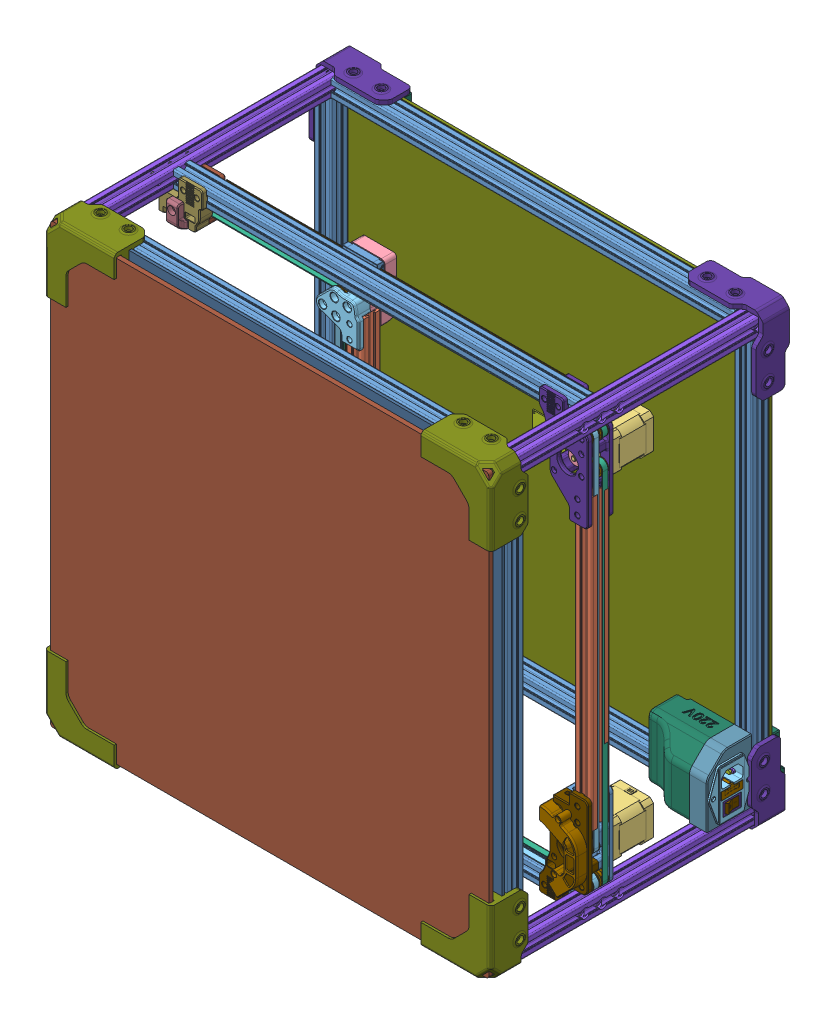
SolidWorks assembly Assem, configuration Default. Lengths in mm. (continued)
Mates (geometry in assembly coordinates): (continued)
- Coincident18: coincident anti-aligned: plane of F695 ZZ (1)^Idler Assembly (1)_1_XY Joint - Right_X Axis_Gantry_VORON2 v2.4 Assembly - Final(2)_VORON2 v2.4 Assembly - Final-1 through (-40.7546 -221.05 -5.3) normal (0 0 1); plane of F695 ZZ (1)^Idler Assembly (1)_1_XY Joint - Right_X Axis_Gantry_VORON2 v2.4 Assembly - Final(2)_VORON2 v2.4 Assembly - Final-2 through (-40.7546 -221.05 -5.3) normal (0 0 -1)
- Concentric9: concentric anti-aligned: cylinder of F695 ZZ (1)^Idler Assembly (1)_1_XY Joint - Right_X Axis_Gantry_VORON2 v2.4 Assembly - Final(2)_VORON2 v2.4 Assembly - Final-1 through (-40.7546 -221.05 -7.3) axis (0 0 1) radius 6.5; cylinder of F695 ZZ (1)^Idler Assembly (1)_1_XY Joint - Right_X Axis_Gantry_VORON2 v2.4 Assembly - Final(2)_VORON2 v2.4 Assembly - Final-2 through (-40.7546 -221.05 -3.3) axis (0 0 -1) radius 6.5
- Concentric10: concentric anti-aligned: cylinder of XY Joint - Right-63^XY Joint - Right_X Axis_Gantry_VORON2 v2.4 Assembly - Final(2)_VORON2 v2.4 Assembly - Final-1 through (-40.7546 -221.05 10.9) axis (0 0 -1) radius 2.7; cylinder of F695 ZZ (1)^Idler Assembly (1)_1_XY Joint - Right_X Axis_Gantry_VORON2 v2.4 Assembly - Final(2)_VORON2 v2.4 Assembly - Final-2 through (-40.7546 -221.05 -5.3) axis (0 0 1) radius 2.5
- Distance7: distance = 1 mm anti-aligned: plane of F695 ZZ (1)^Idler Assembly (1)_1_XY Joint - Right_X Axis_Gantry_VORON2 v2.4 Assembly - Final(2)_VORON2 v2.4 Assembly - Final-1 through (-40.7546 -221.05 -9.3) normal (0 0 -1); plane of XY Joint - Right-63^XY Joint - Right_X Axis_Gantry_VORON2 v2.4 Assembly - Final(2)_VORON2 v2.4 Assembly - Final-1 through (-40.1448 -212.776 -10.3) normal (0 0 1)
- Coincident20: coincident anti-aligned: plane of XY Joint - Right-63^XY Joint - Right_X Axis_Gantry_VORON2 v2.4 Assembly - Final(2)_VORON2 v2.4 Assembly - Final-1 through (-40.1448 -212.776 -10.3) normal (0 0 1); plane of M5 1mm Spacer (1)^Idler Assembly (1)_1_XY Joint - Right_X Axis_Gantry_VORON2 v2.4 Assembly - Final(2)_VORON2 v2.4 Assembly - Final-1 through (-40.7546 -221.05 -10.3) normal (0 0 -1)
- Concentric13: concentric anti-aligned: cylinder of F695 ZZ (1)^Idler Assembly (1)_1_XY Joint - Right_X Axis_Gantry_VORON2 v2.4 Assembly - Final(2)_VORON2 v2.4 Assembly - Final-1 through (-40.7546 -221.05 -9.3) axis (0 0 1) radius 7.5; cylinder of M5 1mm Spacer (1)^Idler Assembly (1)_1_XY Joint - Right_X Axis_Gantry_VORON2 v2.4 Assembly - Final(2)_VORON2 v2.4 Assembly - Final-1 through (-40.7546 -221.05 -9.3) axis (0 0 -1) radius 5
- Coincident21: coincident anti-aligned: plane of F695 ZZ (1)^Idler Assembly (1)_1_XY Joint - Right_X Axis_Gantry_VORON2 v2.4 Assembly - Final(2)_VORON2 v2.4 Assembly - Final-2 through (-40.7546 -221.05 -1.3) normal (0 0 1); plane of M5 1mm Spacer (1)^Idler Assembly (1)_1_XY Joint - Right_X Axis_Gantry_VORON2 v2.4 Assembly - Final(2)_VORON2 v2.4 Assembly - Final-2 through (-40.7546 -221.05 -1.3) normal (0 0 -1)
- Concentric14: concentric aligned: cylinder of F695 ZZ (1)^Idler Assembly (1)_1_XY Joint - Right_X Axis_Gantry_VORON2 v2.4 Assembly - Final(2)_VORON2 v2.4 Assembly - Final-2 through (-40.7546 -221.05 -1.3) axis (0 0 -1) radius 7.5; cylinder of M5 1mm Spacer (1)^Idler Assembly (1)_1_XY Joint - Right_X Axis_Gantry_VORON2 v2.4 Assembly - Final(2)_VORON2 v2.4 Assembly - Final-2 through (-40.7546 -221.05 -0.3) axis (0 0 -1) radius 5
- Distance8: distance = 250 mm aligned: plane of ALP2020_460-1 through (230 250 8.5) normal (0 1 0)
- Coincident23: coincident aligned: plane of ALP2020_460-1 through (0 240 0) normal (1 0 0)
- Coincident24: coincident aligned: plane of ALP2020_460-1 through (0 240 0) normal (0 0 1)
- Concentric15: concentric anti-aligned: cylinder of F695 ZZ (1)^Idler Assembly (1)_1_XY Joint - Right_X Axis_Gantry_VORON2 v2.4 Assembly - Final(2)_VORON2 v2.4 Assembly - Final-3 through (-40.7546 221.05 6.7) axis (0 0 -1) radius 6.5; cylinder of F695 ZZ (1)^Idler Assembly (1)_1_XY Joint - Right_X Axis_Gantry_VORON2 v2.4 Assembly - Final(2)_VORON2 v2.4 Assembly - Final-4 through (-40.7546 221.05 2.7) axis (0 0 1) radius 6.5
- Coincident25: coincident anti-aligned: plane of F695 ZZ (1)^Idler Assembly (1)_1_XY Joint - Right_X Axis_Gantry_VORON2 v2.4 Assembly - Final(2)_VORON2 v2.4 Assembly - Final-3 through (-40.7546 221.05 4.7) normal (0 0 -1); plane of F695 ZZ (1)^Idler Assembly (1)_1_XY Joint - Right_X Axis_Gantry_VORON2 v2.4 Assembly - Final(2)_VORON2 v2.4 Assembly - Final-4 through (-40.7546 221.05 4.7) normal (0 0 1)
- Concentric16: concentric anti-aligned: cylinder of M5 1mm Spacer (1)^Idler Assembly (1)_1_XY Joint - Right_X Axis_Gantry_VORON2 v2.4 Assembly - Final(2)_VORON2 v2.4 Assembly - Final-4 through (-40.7546 221.05 0.7) axis (0 0 -1) radius 5; cylinder of F695 ZZ (1)^Idler Assembly (1)_1_XY Joint - Right_X Axis_Gantry_VORON2 v2.4 Assembly - Final(2)_VORON2 v2.4 Assembly - Final-4 through (-40.7546 221.05 0.7) axis (0 0 1) radius 7.5
- Concentric17: concentric aligned: cylinder of M5 1mm Spacer (1)^Idler Assembly (1)_1_XY Joint - Right_X Axis_Gantry_VORON2 v2.4 Assembly - Final(2)_VORON2 v2.4 Assembly - Final-3 through (-40.7546 221.05 9.7) axis (0 0 -1) radius 5; cylinder of F695 ZZ (1)^Idler Assembly (1)_1_XY Joint - Right_X Axis_Gantry_VORON2 v2.4 Assembly - Final(2)_VORON2 v2.4 Assembly - Final-3 through (-40.7546 221.05 8.7) axis (0 0 -1) radius 7.5
- Coincident26: coincident anti-aligned: plane of M5 1mm Spacer (1)^Idler Assembly (1)_1_XY Joint - Right_X Axis_Gantry_VORON2 v2.4 Assembly - Final(2)_VORON2 v2.4 Assembly - Final-3 through (-40.7546 221.05 8.7) normal (0 0 -1); plane of F695 ZZ (1)^Idler Assembly (1)_1_XY Joint - Right_X Axis_Gantry_VORON2 v2.4 Assembly - Final(2)_VORON2 v2.4 Assembly - Final-3 through (-40.7546 221.05 8.7) normal (0 0 1)
- Concentric18: concentric anti-aligned: cylinder of XY Joint - Left-57^XY Joint - Left_X Axis_Gantry_VORON2 v2.4 Assembly - Final(2)_VORON2 v2.4 Assembly - Final-1 through (-40.7546 221.05 15.7) axis (0 0 1) radius 4.4; cylinder of F695 ZZ (1)^Idler Assembly (1)_1_XY Joint - Right_X Axis_Gantry_VORON2 v2.4 Assembly - Final(2)_VORON2 v2.4 Assembly - Final-4 through (-40.7546 221.05 4.7) axis (0 0 -1) radius 2.5
- Coincident27: coincident anti-aligned: plane of XY Joint - Left-57^XY Joint - Left_X Axis_Gantry_VORON2 v2.4 Assembly - Final(2)_VORON2 v2.4 Assembly - Final-1 through (-42.8669 212.651 9.7) normal (0 0 -1); plane of M5 1mm Spacer (1)^Idler Assembly (1)_1_XY Joint - Right_X Axis_Gantry_VORON2 v2.4 Assembly - Final(2)_VORON2 v2.4 Assembly - Final-3 through (-40.7546 221.05 9.7) normal (0 0 1)
- Coincident28: coincident anti-aligned: plane of M5 1mm Spacer (1)^Idler Assembly (1)_1_XY Joint - Right_X Axis_Gantry_VORON2 v2.4 Assembly - Final(2)_VORON2 v2.4 Assembly - Final-4 through (-40.7546 221.05 0.7) normal (0 0 1); plane of F695 ZZ (1)^Idler Assembly (1)_1_XY Joint - Right_X Axis_Gantry_VORON2 v2.4 Assembly - Final(2)_VORON2 v2.4 Assembly - Final-4 through (-40.7546 221.05 0.7) normal (0 0 -1)
- Coincident29: coincident anti-aligned: plane of Front Idler B Bottom^Front Idler B_Gantry_VORON2 v2.4 Assembly - Final(2)_VORON2 v2.4 Assembly - Final-1 through (-218.2501 228 0) normal (0 0 1); plane of Front Idler B Top^Front Idler B_Gantry_VORON2 v2.4 Assembly - Final(2)_VORON2 v2.4 Assembly - Final-1 through (-207 239.4979 0) normal (0 0 -1)
- Coincident31: coincident aligned: plane of Front Idler B Bottom^Front Idler B_Gantry_VORON2 v2.4 Assembly - Final(2)_VORON2 v2.4 Assembly - Final-1 through (-211.5 218.8388 -15) normal (1 0 0); plane of Front Idler B Top^Front Idler B_Gantry_VORON2 v2.4 Assembly - Final(2)_VORON2 v2.4 Assembly - Final-1 through (-211.5 218.8388 -15) normal (1 0 0)
- Coincident33: coincident anti-aligned: plane of ALP2020_450-1 through (230 231.5 10) normal (0 0 1); plane of Front Idler B Top^Front Idler B_Gantry_VORON2 v2.4 Assembly - Final(2)_VORON2 v2.4 Assembly - Final-1 through (-208.3 228 10) normal (0 0 -1)
- Distance9: distance = 10 mm aligned: plane of Front Idler B Top^Front Idler B_Gantry_VORON2 v2.4 Assembly - Final(2)_VORON2 v2.4 Assembly - Final-1 through (-220 229 10) normal (-1 0 0); plane of ALP2020_450-1 through (-230 245.9 -2.0109) normal (-1 0 0)
- Coincident35: coincident aligned: plane of ALP2020_450-1 through (230 250 8.5) normal (0 1 0); plane of Front Idler B Top^Front Idler B_Gantry_VORON2 v2.4 Assembly - Final(2)_VORON2 v2.4 Assembly - Final-1 through (-221.6 250 10) normal (0 1 0)
- Coincident36: coincident aligned: plane of Front Idler B Bottom^Front Idler B_Gantry_VORON2 v2.4 Assembly - Final(2)_VORON2 v2.4 Assembly - Final-1 through (-221.6 250 -15) normal (0 1 0); plane of Front Idler B Top^Front Idler B_Gantry_VORON2 v2.4 Assembly - Final(2)_VORON2 v2.4 Assembly - Final-1 through (-221.6 250 10) normal (0 1 0)
- Coincident38: coincident anti-aligned: plane of F695 ZZ (1)^Idler Assembly (1)_1_XY Joint - Right_X Axis_Gantry_VORON2 v2.4 Assembly - Final(2)_VORON2 v2.4 Assembly - Final-5 through (-219.5002 221.0003 -5) normal (0 0 -1); plane of F695 ZZ (1)^Idler Assembly (1)_1_XY Joint - Right_X Axis_Gantry_VORON2 v2.4 Assembly - Final(2)_VORON2 v2.4 Assembly - Final-6 through (-219.5002 221.0003 -5) normal (0 0 1)
- Concentric23: concentric anti-aligned: cylinder of F695 ZZ (1)^Idler Assembly (1)_1_XY Joint - Right_X Axis_Gantry_VORON2 v2.4 Assembly - Final(2)_VORON2 v2.4 Assembly - Final-5 through (-219.5002 221.0003 -3) axis (0 0 -1) radius 6.5; cylinder of F695 ZZ (1)^Idler Assembly (1)_1_XY Joint - Right_X Axis_Gantry_VORON2 v2.4 Assembly - Final(2)_VORON2 v2.4 Assembly - Final-6 through (-219.5002 221.0003 -7) axis (0 0 1) radius 6.5
- Concentric24: concentric anti-aligned: cylinder of F695 ZZ (1)^Idler Assembly (1)_1_XY Joint - Right_X Axis_Gantry_VORON2 v2.4 Assembly - Final(2)_VORON2 v2.4 Assembly - Final-5 through (-219.5002 221.0003 -1) axis (0 0 -1) radius 7.5; cylinder of M5 1mm Spacer (1)^Idler Assembly (1)_1_XY Joint - Right_X Axis_Gantry_VORON2 v2.4 Assembly - Final(2)_VORON2 v2.4 Assembly - Final-6 through (-219.5002 221.0003 -1) axis (0 0 1) radius 5
- Coincident39: coincident anti-aligned: plane of F695 ZZ (1)^Idler Assembly (1)_1_XY Joint - Right_X Axis_Gantry_VORON2 v2.4 Assembly - Final(2)_VORON2 v2.4 Assembly - Final-5 through (-219.5002 221.0003 -1) normal (0 0 1); plane of M5 1mm Spacer (1)^Idler Assembly (1)_1_XY Joint - Right_X Axis_Gantry_VORON2 v2.4 Assembly - Final(2)_VORON2 v2.4 Assembly - Final-6 through (-219.5002 221.0003 -1) normal (0 0 -1)
- Coincident40: coincident anti-aligned: plane of M5 1mm Spacer (1)^Idler Assembly (1)_1_XY Joint - Right_X Axis_Gantry_VORON2 v2.4 Assembly - Final(2)_VORON2 v2.4 Assembly - Final-5 through (-219.5002 221.0003 -9) normal (0 0 1); plane of F695 ZZ (1)^Idler Assembly (1)_1_XY Joint - Right_X Axis_Gantry_VORON2 v2.4 Assembly - Final(2)_VORON2 v2.4 Assembly - Final-6 through (-219.5002 221.0003 -9) normal (0 0 -1)
- Concentric25: concentric aligned: cylinder of M5 1mm Spacer (1)^Idler Assembly (1)_1_XY Joint - Right_X Axis_Gantry_VORON2 v2.4 Assembly - Final(2)_VORON2 v2.4 Assembly - Final-5 through (-219.5002 221.0003 -10) axis (0 0 1) radius 5; cylinder of F695 ZZ (1)^Idler Assembly (1)_1_XY Joint - Right_X Axis_Gantry_VORON2 v2.4 Assembly - Final(2)_VORON2 v2.4 Assembly - Final-6 through (-219.5002 221.0003 -9) axis (0 0 1) radius 7.5
- Concentric26: concentric anti-aligned: cylinder of Tensioner B-26^Tensioner B_Front Idler B_Gantry_VORON2 v2.4 Assembly - Final(2)_VORON2 v2.4 Assembly - Final-1 through (-219.5002 221.0003 -15) axis (0 0 1) radius 2.7; cylinder of F695 ZZ (1)^Idler Assembly (1)_1_XY Joint - Right_X Axis_Gantry_VORON2 v2.4 Assembly - Final(2)_VORON2 v2.4 Assembly - Final-6 through (-219.5002 221.0003 -5) axis (0 0 -1) radius 2.5
- Coincident42: coincident anti-aligned: plane of Front Idler A Bottom (1)^Front Idler A_Gantry_VORON2 v2.4 Assembly - Final(2)_VORON2 v2.4 Assembly - Final-1 through (-244.5002 -212 0) normal (0 0 1); plane of Front Idler A Top^Front Idler A_Gantry_VORON2 v2.4 Assembly - Final(2)_VORON2 v2.4 Assembly - Final-1 through (-218.2501 -228 0) normal (0 0 -1)
- Coincident43: coincident aligned: plane of Front Idler A Bottom (1)^Front Idler A_Gantry_VORON2 v2.4 Assembly - Final(2)_VORON2 v2.4 Assembly - Final-1 through (-221.6 -250 -15) normal (0 -1 0); plane of Front Idler A Top^Front Idler A_Gantry_VORON2 v2.4 Assembly - Final(2)_VORON2 v2.4 Assembly - Final-1 through (-221.6 -250 10) normal (0 -1 0)
- Coincident44: coincident aligned: plane of Front Idler A Bottom (1)^Front Idler A_Gantry_VORON2 v2.4 Assembly - Final(2)_VORON2 v2.4 Assembly - Final-1 through (-220 -229 -15) normal (-1 0 0); plane of Front Idler A Top^Front Idler A_Gantry_VORON2 v2.4 Assembly - Final(2)_VORON2 v2.4 Assembly - Final-1 through (-220 -229 10) normal (-1 0 0)
- Coincident45: coincident aligned: plane of ALP2020_450-2 through (230 -250 3.9) normal (0 -1 0); plane of Front Idler A Top^Front Idler A_Gantry_VORON2 v2.4 Assembly - Final(2)_VORON2 v2.4 Assembly - Final-1 through (-221.6 -250 10) normal (0 -1 0)
- Coincident46: coincident anti-aligned: plane of ALP2020_450-2 through (230 -248.5 10) normal (0 0 1); plane of Front Idler A Top^Front Idler A_Gantry_VORON2 v2.4 Assembly - Final(2)_VORON2 v2.4 Assembly - Final-1 through (-208.3 -228 10) normal (0 0 -1)
- Distance10: distance = 10 mm aligned: plane of ALP2020_450-2 through (-230 -234.1 -2.0109) normal (-1 0 0); plane of Front Idler A Top^Front Idler A_Gantry_VORON2 v2.4 Assembly - Final(2)_VORON2 v2.4 Assembly - Final-1 through (-220 -229 10) normal (-1 0 0)
- Concentric28: concentric anti-aligned: cylinder of Front Idler A Bottom (1)^Front Idler A_Gantry_VORON2 v2.4 Assembly - Final(2)_VORON2 v2.4 Assembly - Final-1 through (-244.5002 -208 0) axis (1 0 0) radius 1.6; cylinder of Tensioner A-25^Tensioner A_Front Idler A_Gantry_VORON2 v2.4 Assembly - Final(2)_VORON2 v2.4 Assembly - Final-1 through (-208.5 -208 0) axis (-1 0 0) radius 2.35
- Coincident48: coincident aligned: plane of Front Idler A Bottom (1)^Front Idler A_Gantry_VORON2 v2.4 Assembly - Final(2)_VORON2 v2.4 Assembly - Final-1 through (-226.5001 -204 0) normal (0 1 0); plane of Tensioner A-25^Tensioner A_Front Idler A_Gantry_VORON2 v2.4 Assembly - Final(2)_VORON2 v2.4 Assembly - Final-1 through (-212.5 -204 15) normal (0 1 0)
- Concentric30: concentric anti-aligned: cylinder of Front Idler B Bottom^Front Idler B_Gantry_VORON2 v2.4 Assembly - Final(2)_VORON2 v2.4 Assembly - Final-1 through (-244.5002 208 0) axis (1 0 0) radius 1.6; cylinder of Tensioner B-26^Tensioner B_Front Idler B_Gantry_VORON2 v2.4 Assembly - Final(2)_VORON2 v2.4 Assembly - Final-1 through (-208.5 208 0) axis (-1 0 0) radius 2.35
- Coincident50: coincident aligned: plane of Front Idler B Top^Front Idler B_Gantry_VORON2 v2.4 Assembly - Final(2)_VORON2 v2.4 Assembly - Final-1 through (-226.5001 204 0) normal (0 -1 0); plane of Tensioner B-26^Tensioner B_Front Idler B_Gantry_VORON2 v2.4 Assembly - Final(2)_VORON2 v2.4 Assembly - Final-1 through (-212.5 204 15) normal (0 -1 0)
- Concentric31: concentric anti-aligned: cylinder of Front Idler B Top^Front Idler B_Gantry_VORON2 v2.4 Assembly - Final(2)_VORON2 v2.4 Assembly - Final-1 through (-219.5002 221.0003 15) axis (0 0 -1) radius 2.6; cylinder of Tensioner B-26^Tensioner B_Front Idler B_Gantry_VORON2 v2.4 Assembly - Final(2)_VORON2 v2.4 Assembly - Final-1 through (-219.5002 221.0003 22.4) axis (0 0 1) radius 4.5
- Coincident51: coincident anti-aligned: plane of F695 ZZ (1)^Idler Assembly (1)_1_XY Joint - Right_X Axis_Gantry_VORON2 v2.4 Assembly - Final(2)_VORON2 v2.4 Assembly - Final-7 through (-219.5002 -221.0003 5) normal (0 0 1); plane of F695 ZZ (1)^Idler Assembly (1)_1_XY Joint - Right_X Axis_Gantry_VORON2 v2.4 Assembly - Final(2)_VORON2 v2.4 Assembly - Final-8 through (-219.5002 -221.0003 5) normal (0 0 -1)
- Concentric32: concentric anti-aligned: cylinder of F695 ZZ (1)^Idler Assembly (1)_1_XY Joint - Right_X Axis_Gantry_VORON2 v2.4 Assembly - Final(2)_VORON2 v2.4 Assembly - Final-7 through (-219.5002 -221.0003 3) axis (0 0 1) radius 6.5; cylinder of F695 ZZ (1)^Idler Assembly (1)_1_XY Joint - Right_X Axis_Gantry_VORON2 v2.4 Assembly - Final(2)_VORON2 v2.4 Assembly - Final-8 through (-219.5002 -221.0003 7) axis (0 0 -1) radius 6.5
- Coincident52: coincident anti-aligned: plane of F695 ZZ (1)^Idler Assembly (1)_1_XY Joint - Right_X Axis_Gantry_VORON2 v2.4 Assembly - Final(2)_VORON2 v2.4 Assembly - Final-7 through (-219.5002 -221.0003 1) normal (0 0 -1); plane of M5 1mm Spacer (1)^Idler Assembly (1)_1_XY Joint - Right_X Axis_Gantry_VORON2 v2.4 Assembly - Final(2)_VORON2 v2.4 Assembly - Final-8 through (-219.5002 -221.0003 1) normal (0 0 1)
- Concentric33: concentric anti-aligned: cylinder of M5 1mm Spacer (1)^Idler Assembly (1)_1_XY Joint - Right_X Axis_Gantry_VORON2 v2.4 Assembly - Final(2)_VORON2 v2.4 Assembly - Final-7 through (-219.5002 -221.0003 9) axis (0 0 1) radius 5; cylinder of F695 ZZ (1)^Idler Assembly (1)_1_XY Joint - Right_X Axis_Gantry_VORON2 v2.4 Assembly - Final(2)_VORON2 v2.4 Assembly - Final-8 through (-219.5002 -221.0003 9) axis (0 0 -1) radius 7.5
- Coincident53: coincident anti-aligned: plane of M5 1mm Spacer (1)^Idler Assembly (1)_1_XY Joint - Right_X Axis_Gantry_VORON2 v2.4 Assembly - Final(2)_VORON2 v2.4 Assembly - Final-7 through (-219.5002 -221.0003 9) normal (0 0 -1); plane of F695 ZZ (1)^Idler Assembly (1)_1_XY Joint - Right_X Axis_Gantry_VORON2 v2.4 Assembly - Final(2)_VORON2 v2.4 Assembly - Final-8 through (-219.5002 -221.0003 9) normal (0 0 1)
- Concentric34: concentric aligned: cylinder of F695 ZZ (1)^Idler Assembly (1)_1_XY Joint - Right_X Axis_Gantry_VORON2 v2.4 Assembly - Final(2)_VORON2 v2.4 Assembly - Final-7 through (-219.5002 -221.0003 1) axis (0 0 1) radius 7.5; cylinder of M5 1mm Spacer (1)^Idler Assembly (1)_1_XY Joint - Right_X Axis_Gantry_VORON2 v2.4 Assembly - Final(2)_VORON2 v2.4 Assembly - Final-8 through (-219.5002 -221.0003 0) axis (0 0 1) radius 5
- Concentric35: concentric aligned: cylinder of Tensioner A-25^Tensioner A_Front Idler A_Gantry_VORON2 v2.4 Assembly - Final(2)_VORON2 v2.4 Assembly - Final-1 through (-219.5002 -221.0003 15) axis (0 0 1) radius 2.7; cylinder of F695 ZZ (1)^Idler Assembly (1)_1_XY Joint - Right_X Axis_Gantry_VORON2 v2.4 Assembly - Final(2)_VORON2 v2.4 Assembly - Final-8 through (-219.5002 -221.0003 5) axis (0 0 1) radius 2.5
- Coincident54: coincident anti-aligned: plane of Front Idler A Top^Front Idler A_Gantry_VORON2 v2.4 Assembly - Final(2)_VORON2 v2.4 Assembly - Final-1 through (-208.3 -228 10) normal (0 0 -1); plane of M5 1mm Spacer (1)^Idler Assembly (1)_1_XY Joint - Right_X Axis_Gantry_VORON2 v2.4 Assembly - Final(2)_VORON2 v2.4 Assembly - Final-7 through (-219.5002 -221.0003 10) normal (0 0 1)
- Concentric36: concentric anti-aligned: cylinder of Front Idler A Top^Front Idler A_Gantry_VORON2 v2.4 Assembly - Final(2)_VORON2 v2.4 Assembly - Final-1 through (-219.5002 -221.0003 -15) axis (0 0 1) radius 2.6; cylinder of Tensioner A-25^Tensioner A_Front Idler A_Gantry_VORON2 v2.4 Assembly - Final(2)_VORON2 v2.4 Assembly - Final-1 through (-219.5002 -221.0003 22.4) axis (0 0 -1) radius 4.5
- Coincident55: coincident anti-aligned: plane of ALP2020_450-1 through (230 243.9 10) normal (0 0 1); plane of B Drive Frame (1)^B Drive_Gantry_VORON2 v2.4 Assembly - Final(2)_VORON2 v2.4 Assembly - Final-1 through (220.1397 181.8752 10) normal (0 0 -1)
- Coincident56: coincident aligned: plane of ALP2020_450-1 through (230 250 8.5) normal (0 1 0); plane of B Drive Frame (1)^B Drive_Gantry_VORON2 v2.4 Assembly - Final(2)_VORON2 v2.4 Assembly - Final-1 through (192.25 250 10) normal (0 1 0)
- Distance11: distance = 10 mm aligned: plane of B Drive Frame (1)^B Drive_Gantry_VORON2 v2.4 Assembly - Final(2)_VORON2 v2.4 Assembly - Final-1 through (220 250 10) normal (1 0 0); plane of ALP2020_450-1 through (230 245.9 -2.0109) normal (1 0 0)
- Coincident58: coincident anti-aligned: plane of A Drive Frame-23^A Drive Frame_A Drive_Gantry_VORON2 v2.4 Assembly - Final(2)_VORON2 v2.4 Assembly - Final-1 through (220.0147 -181.8367 0) normal (0 0 -1); plane of A Drive Frame-24^A Drive Frame_A Drive_Gantry_VORON2 v2.4 Assembly - Final(2)_VORON2 v2.4 Assembly - Final-1 through (221.5147 -186.0931 0) normal (0 0 1)
- Coincident59: coincident aligned: plane of A Drive Frame-23^A Drive Frame_A Drive_Gantry_VORON2 v2.4 Assembly - Final(2)_VORON2 v2.4 Assembly - Final-1 through (192.25 -250 10) normal (0 -1 0); plane of A Drive Frame-24^A Drive Frame_A Drive_Gantry_VORON2 v2.4 Assembly - Final(2)_VORON2 v2.4 Assembly - Final-1 through (192.25 -250 -16.6) normal (0 -1 0)
- Coincident61: coincident aligned: plane of A Drive Frame-23^A Drive Frame_A Drive_Gantry_VORON2 v2.4 Assembly - Final(2)_VORON2 v2.4 Assembly - Final-1 through (248.0294 -221.1733 10) normal (1 0 0); plane of A Drive Frame-24^A Drive Frame_A Drive_Gantry_VORON2 v2.4 Assembly - Final(2)_VORON2 v2.4 Assembly - Final-1 through (248.0294 -221.1733 -16.6) normal (1 0 0)
- Coincident64: coincident anti-aligned: plane of ALP2020_450-2 through (230 -248.5 10) normal (0 0 1); plane of A Drive Frame-23^A Drive Frame_A Drive_Gantry_VORON2 v2.4 Assembly - Final(2)_VORON2 v2.4 Assembly - Final-1 through (220.1397 -181.8752 10) normal (0 0 -1)
- Coincident65: coincident aligned: plane of ALP2020_450-2 through (230 -250 3.9) normal (0 -1 0); plane of A Drive Frame-23^A Drive Frame_A Drive_Gantry_VORON2 v2.4 Assembly - Final(2)_VORON2 v2.4 Assembly - Final-1 through (192.25 -250 10) normal (0 -1 0)
- Distance12: distance = 10 mm aligned: plane of A Drive Frame-23^A Drive Frame_A Drive_Gantry_VORON2 v2.4 Assembly - Final(2)_VORON2 v2.4 Assembly - Final-1 through (220 -250 10) normal (1 0 0); plane of ALP2020_450-2 through (230 -234.1 -2.0109) normal (1 0 0)
- Coincident67: coincident anti-aligned: plane of A Drive Frame-23^A Drive Frame_A Drive_Gantry_VORON2 v2.4 Assembly - Final(2)_VORON2 v2.4 Assembly - Final-1 through (220.1397 -181.8752 10) normal (0 0 -1); plane of ALP2020_330-1 through (246.5294 164.9774 10) normal (0 0 1)
- Coincident68: coincident aligned: plane of A Drive Frame-23^A Drive Frame_A Drive_Gantry_VORON2 v2.4 Assembly - Final(2)_VORON2 v2.4 Assembly - Final-1 through (248.0294 -221.1733 10) normal (1 0 0); plane of ALP2020_330-1 through (248.0294 164.9774 3.9) normal (1 0 0)
- Distance13: distance = 5 mm anti-aligned: plane of ALP2020_330-1 through (232.1294 164.9774 -2.0109) normal (0 1 0); plane of B Drive Frame (1)^B Drive_Gantry_VORON2 v2.4 Assembly - Final(2)_VORON2 v2.4 Assembly - Final-1 through (242.029 169.9774 0) normal (0 -1 0)
- Concentric37: concentric aligned: cylinder of M5 1mm Spacer (1)^Idler Assembly (1)_1_XY Joint - Right_X Axis_Gantry_VORON2 v2.4 Assembly - Final(2)_VORON2 v2.4 Assembly - Final-9 through (240.5294 -221.1733 0) axis (0 0 1) radius 5; cylinder of F695 ZZ (1)^Idler Assembly (1)_1_XY Joint - Right_X Axis_Gantry_VORON2 v2.4 Assembly - Final(2)_VORON2 v2.4 Assembly - Final-10 through (240.5294 -221.1733 1) axis (0 0 1) radius 7.5
- Coincident70: coincident anti-aligned: plane of F695 ZZ (1)^Idler Assembly (1)_1_XY Joint - Right_X Axis_Gantry_VORON2 v2.4 Assembly - Final(2)_VORON2 v2.4 Assembly - Final-9 through (240.5294 -221.1733 5) normal (0 0 -1); plane of F695 ZZ (1)^Idler Assembly (1)_1_XY Joint - Right_X Axis_Gantry_VORON2 v2.4 Assembly - Final(2)_VORON2 v2.4 Assembly - Final-10 through (240.5294 -221.1733 5) normal (0 0 1)
- Concentric38: concentric anti-aligned: cylinder of F695 ZZ (1)^Idler Assembly (1)_1_XY Joint - Right_X Axis_Gantry_VORON2 v2.4 Assembly - Final(2)_VORON2 v2.4 Assembly - Final-9 through (240.5294 -221.1733 7) axis (0 0 -1) radius 6.5; cylinder of F695 ZZ (1)^Idler Assembly (1)_1_XY Joint - Right_X Axis_Gantry_VORON2 v2.4 Assembly - Final(2)_VORON2 v2.4 Assembly - Final-10 through (240.5294 -221.1733 3) axis (0 0 1) radius 6.5
- Concentric39: concentric anti-aligned: cylinder of F695 ZZ (1)^Idler Assembly (1)_1_XY Joint - Right_X Axis_Gantry_VORON2 v2.4 Assembly - Final(2)_VORON2 v2.4 Assembly - Final-9 through (240.5294 -221.1733 9) axis (0 0 -1) radius 7.5; cylinder of M5 1mm Spacer (1)^Idler Assembly (1)_1_XY Joint - Right_X Axis_Gantry_VORON2 v2.4 Assembly - Final(2)_VORON2 v2.4 Assembly - Final-10 through (240.5294 -221.1733 9) axis (0 0 1) radius 5
- Coincident71: coincident anti-aligned: plane of M5 1mm Spacer (1)^Idler Assembly (1)_1_XY Joint - Right_X Axis_Gantry_VORON2 v2.4 Assembly - Final(2)_VORON2 v2.4 Assembly - Final-9 through (240.5294 -221.1733 1) normal (0 0 1); plane of F695 ZZ (1)^Idler Assembly (1)_1_XY Joint - Right_X Axis_Gantry_VORON2 v2.4 Assembly - Final(2)_VORON2 v2.4 Assembly - Final-10 through (240.5294 -221.1733 1) normal (0 0 -1)
- Coincident72: coincident anti-aligned: plane of F695 ZZ (1)^Idler Assembly (1)_1_XY Joint - Right_X Axis_Gantry_VORON2 v2.4 Assembly - Final(2)_VORON2 v2.4 Assembly - Final-9 through (240.5294 -221.1733 9) normal (0 0 1); plane of M5 1mm Spacer (1)^Idler Assembly (1)_1_XY Joint - Right_X Axis_Gantry_VORON2 v2.4 Assembly - Final(2)_VORON2 v2.4 Assembly - Final-10 through (240.5294 -221.1733 9) normal (0 0 -1)
- Concentric40: concentric anti-aligned: cylinder of F695 ZZ (1)^Idler Assembly (1)_1_XY Joint - Right_X Axis_Gantry_VORON2 v2.4 Assembly - Final(2)_VORON2 v2.4 Assembly - Final-11 through (240.5294 -221.1733 -7) axis (0 0 1) radius 6.5; cylinder of F695 ZZ (1)^Idler Assembly (1)_1_XY Joint - Right_X Axis_Gantry_VORON2 v2.4 Assembly - Final(2)_VORON2 v2.4 Assembly - Final-12 through (240.5294 -221.1733 -3) axis (0 0 -1) radius 6.5
- Concentric41: concentric aligned: cylinder of F695 ZZ (1)^Idler Assembly (1)_1_XY Joint - Right_X Axis_Gantry_VORON2 v2.4 Assembly - Final(2)_VORON2 v2.4 Assembly - Final-11 through (240.5294 -221.1733 -9) axis (0 0 1) radius 7.5; cylinder of M5 1mm Spacer (1)^Idler Assembly (1)_1_XY Joint - Right_X Axis_Gantry_VORON2 v2.4 Assembly - Final(2)_VORON2 v2.4 Assembly - Final-12 through (240.5294 -221.1733 -10) axis (0 0 1) radius 5
- Coincident73: coincident anti-aligned: plane of F695 ZZ (1)^Idler Assembly (1)_1_XY Joint - Right_X Axis_Gantry_VORON2 v2.4 Assembly - Final(2)_VORON2 v2.4 Assembly - Final-11 through (240.5294 -221.1733 -5) normal (0 0 1); plane of F695 ZZ (1)^Idler Assembly (1)_1_XY Joint - Right_X Axis_Gantry_VORON2 v2.4 Assembly - Final(2)_VORON2 v2.4 Assembly - Final-12 through (240.5294 -221.1733 -5) normal (0 0 -1)
- Concentric42: concentric anti-aligned: cylinder of M5 1mm Spacer (1)^Idler Assembly (1)_1_XY Joint - Right_X Axis_Gantry_VORON2 v2.4 Assembly - Final(2)_VORON2 v2.4 Assembly - Final-11 through (240.5294 -221.1733 -1) axis (0 0 1) radius 5; cylinder of F695 ZZ (1)^Idler Assembly (1)_1_XY Joint - Right_X Axis_Gantry_VORON2 v2.4 Assembly - Final(2)_VORON2 v2.4 Assembly - Final-12 through (240.5294 -221.1733 -1) axis (0 0 -1) radius 7.5
- Coincident74: coincident anti-aligned: plane of F695 ZZ (1)^Idler Assembly (1)_1_XY Joint - Right_X Axis_Gantry_VORON2 v2.4 Assembly - Final(2)_VORON2 v2.4 Assembly - Final-11 through (240.5294 -221.1733 -9) normal (0 0 -1); plane of M5 1mm Spacer (1)^Idler Assembly (1)_1_XY Joint - Right_X Axis_Gantry_VORON2 v2.4 Assembly - Final(2)_VORON2 v2.4 Assembly - Final-12 through (240.5294 -221.1733 -9) normal (0 0 1)
- Coincident75: coincident anti-aligned: plane of M5 1mm Spacer (1)^Idler Assembly (1)_1_XY Joint - Right_X Axis_Gantry_VORON2 v2.4 Assembly - Final(2)_VORON2 v2.4 Assembly - Final-11 through (240.5294 -221.1733 -1) normal (0 0 -1); plane of F695 ZZ (1)^Idler Assembly (1)_1_XY Joint - Right_X Axis_Gantry_VORON2 v2.4 Assembly - Final(2)_VORON2 v2.4 Assembly - Final-12 through (240.5294 -221.1733 -1) normal (0 0 1)
- Coincident76: coincident anti-aligned: plane of M5 1mm Spacer (1)^Idler Assembly (1)_1_XY Joint - Right_X Axis_Gantry_VORON2 v2.4 Assembly - Final(2)_VORON2 v2.4 Assembly - Final-9 through (240.5294 -221.1733 0) normal (0 0 -1); plane of M5 1mm Spacer (1)^Idler Assembly (1)_1_XY Joint - Right_X Axis_Gantry_VORON2 v2.4 Assembly - Final(2)_VORON2 v2.4 Assembly - Final-11 through (240.5294 -221.1733 0) normal (0 0 1)
- Concentric43: concentric aligned: cylinder of F695 ZZ (1)^Idler Assembly (1)_1_XY Joint - Right_X Axis_Gantry_VORON2 v2.4 Assembly - Final(2)_VORON2 v2.4 Assembly - Final-10 through (240.5294 -221.1733 5) axis (0 0 -1) radius 2.5; cylinder of F695 ZZ (1)^Idler Assembly (1)_1_XY Joint - Right_X Axis_Gantry_VORON2 v2.4 Assembly - Final(2)_VORON2 v2.4 Assembly - Final-11 through (240.5294 -221.1733 -5) axis (0 0 -1) radius 2.5
- Concentric44: concentric aligned: cylinder of A Drive Frame-23^A Drive Frame_A Drive_Gantry_VORON2 v2.4 Assembly - Final(2)_VORON2 v2.4 Assembly - Final-1 through (240.5294 -221.1733 15) axis (0 0 -1) radius 2.7; cylinder of F695 ZZ (1)^Idler Assembly (1)_1_XY Joint - Right_X Axis_Gantry_VORON2 v2.4 Assembly - Final(2)_VORON2 v2.4 Assembly - Final-11 through (240.5294 -221.1733 -5) axis (0 0 -1) radius 2.5
- Coincident77: coincident anti-aligned: plane of A Drive Frame-24^A Drive Frame_A Drive_Gantry_VORON2 v2.4 Assembly - Final(2)_VORON2 v2.4 Assembly - Final-1 through (220.0147 -181.8367 -10) normal (0 0 1); plane of M5 1mm Spacer (1)^Idler Assembly (1)_1_XY Joint - Right_X Axis_Gantry_VORON2 v2.4 Assembly - Final(2)_VORON2 v2.4 Assembly - Final-12 through (240.5294 -221.1733 -10) normal (0 0 -1)
- Concentric45: concentric anti-aligned: cylinder of F695 ZZ (1)^Idler Assembly (1)_1_XY Joint - Right_X Axis_Gantry_VORON2 v2.4 Assembly - Final(2)_VORON2 v2.4 Assembly - Final-13 through (240.5294 221.1733 -3) axis (0 0 -1) radius 6.5; cylinder of F695 ZZ (1)^Idler Assembly (1)_1_XY Joint - Right_X Axis_Gantry_VORON2 v2.4 Assembly - Final(2)_VORON2 v2.4 Assembly - Final-14 through (240.5294 221.1733 -7) axis (0 0 1) radius 6.5
- Coincident78: coincident anti-aligned: plane of M5 1mm Spacer (1)^Idler Assembly (1)_1_XY Joint - Right_X Axis_Gantry_VORON2 v2.4 Assembly - Final(2)_VORON2 v2.4 Assembly - Final-13 through (240.5294 221.1733 -9) normal (0 0 1); plane of F695 ZZ (1)^Idler Assembly (1)_1_XY Joint - Right_X Axis_Gantry_VORON2 v2.4 Assembly - Final(2)_VORON2 v2.4 Assembly - Final-14 through (240.5294 221.1733 -9) normal (0 0 -1)
- Concentric46: concentric anti-aligned: cylinder of F695 ZZ (1)^Idler Assembly (1)_1_XY Joint - Right_X Axis_Gantry_VORON2 v2.4 Assembly - Final(2)_VORON2 v2.4 Assembly - Final-13 through (240.5294 221.1733 -1) axis (0 0 -1) radius 7.5; cylinder of M5 1mm Spacer (1)^Idler Assembly (1)_1_XY Joint - Right_X Axis_Gantry_VORON2 v2.4 Assembly - Final(2)_VORON2 v2.4 Assembly - Final-14 through (240.5294 221.1733 -1) axis (0 0 1) radius 5
- Coincident79: coincident anti-aligned: plane of F695 ZZ (1)^Idler Assembly (1)_1_XY Joint - Right_X Axis_Gantry_VORON2 v2.4 Assembly - Final(2)_VORON2 v2.4 Assembly - Final-13 through (240.5294 221.1733 -5) normal (0 0 -1); plane of F695 ZZ (1)^Idler Assembly (1)_1_XY Joint - Right_X Axis_Gantry_VORON2 v2.4 Assembly - Final(2)_VORON2 v2.4 Assembly - Final-14 through (240.5294 221.1733 -5) normal (0 0 1)
- Concentric47: concentric aligned: cylinder of M5 1mm Spacer (1)^Idler Assembly (1)_1_XY Joint - Right_X Axis_Gantry_VORON2 v2.4 Assembly - Final(2)_VORON2 v2.4 Assembly - Final-13 through (240.5294 221.1733 -10) axis (0 0 1) radius 5; cylinder of F695 ZZ (1)^Idler Assembly (1)_1_XY Joint - Right_X Axis_Gantry_VORON2 v2.4 Assembly - Final(2)_VORON2 v2.4 Assembly - Final-14 through (240.5294 221.1733 -9) axis (0 0 1) radius 7.5
- Coincident80: coincident anti-aligned: plane of F695 ZZ (1)^Idler Assembly (1)_1_XY Joint - Right_X Axis_Gantry_VORON2 v2.4 Assembly - Final(2)_VORON2 v2.4 Assembly - Final-13 through (240.5294 221.1733 -1) normal (0 0 1); plane of M5 1mm Spacer (1)^Idler Assembly (1)_1_XY Joint - Right_X Axis_Gantry_VORON2 v2.4 Assembly - Final(2)_VORON2 v2.4 Assembly - Final-14 through (240.5294 221.1733 -1) normal (0 0 -1)
- Coincident81: coincident anti-aligned: plane of M5 1mm Spacer (1)^Idler Assembly (1)_1_XY Joint - Right_X Axis_Gantry_VORON2 v2.4 Assembly - Final(2)_VORON2 v2.4 Assembly - Final-14 through (240.5294 221.1733 0) normal (0 0 1); plane of M5 1mm Spacer (1)^Idler Assembly (1)_1_XY Joint - Right_X Axis_Gantry_VORON2 v2.4 Assembly - Final(2)_VORON2 v2.4 Assembly - Final-16 through (240.5294 221.1733 0) normal (0 0 -1)
- Concentric48: concentric aligned: cylinder of F695 ZZ (1)^Idler Assembly (1)_1_XY Joint - Right_X Axis_Gantry_VORON2 v2.4 Assembly - Final(2)_VORON2 v2.4 Assembly - Final-14 through (240.5294 221.1733 -5) axis (0 0 -1) radius 2.5; cylinder of F695 ZZ (1)^Idler Assembly (1)_1_XY Joint - Right_X Axis_Gantry_VORON2 v2.4 Assembly - Final(2)_VORON2 v2.4 Assembly - Final-15 through (240.5294 221.1733 5) axis (0 0 -1) radius 2.5
- Concentric49: concentric anti-aligned: cylinder of F695 ZZ (1)^Idler Assembly (1)_1_XY Joint - Right_X Axis_Gantry_VORON2 v2.4 Assembly - Final(2)_VORON2 v2.4 Assembly - Final-15 through (240.5294 221.1733 3) axis (0 0 1) radius 6.5; cylinder of F695 ZZ (1)^Idler Assembly (1)_1_XY Joint - Right_X Axis_Gantry_VORON2 v2.4 Assembly - Final(2)_VORON2 v2.4 Assembly - Final-16 through (240.5294 221.1733 7) axis (0 0 -1) radius 6.5
- Concentric50: concentric aligned: cylinder of F695 ZZ (1)^Idler Assembly (1)_1_XY Joint - Right_X Axis_Gantry_VORON2 v2.4 Assembly - Final(2)_VORON2 v2.4 Assembly - Final-15 through (240.5294 221.1733 1) axis (0 0 1) radius 7.5; cylinder of M5 1mm Spacer (1)^Idler Assembly (1)_1_XY Joint - Right_X Axis_Gantry_VORON2 v2.4 Assembly - Final(2)_VORON2 v2.4 Assembly - Final-16 through (240.5294 221.1733 0) axis (0 0 1) radius 5
- Coincident82: coincident anti-aligned: plane of F695 ZZ (1)^Idler Assembly (1)_1_XY Joint - Right_X Axis_Gantry_VORON2 v2.4 Assembly - Final(2)_VORON2 v2.4 Assembly - Final-15 through (240.5294 221.1733 5) normal (0 0 1); plane of F695 ZZ (1)^Idler Assembly (1)_1_XY Joint - Right_X Axis_Gantry_VORON2 v2.4 Assembly - Final(2)_VORON2 v2.4 Assembly - Final-16 through (240.5294 221.1733 5) normal (0 0 -1)
- Concentric51: concentric anti-aligned: cylinder of M5 1mm Spacer (1)^Idler Assembly (1)_1_XY Joint - Right_X Axis_Gantry_VORON2 v2.4 Assembly - Final(2)_VORON2 v2.4 Assembly - Final-15 through (240.5294 221.1733 9) axis (0 0 1) radius 5; cylinder of F695 ZZ (1)^Idler Assembly (1)_1_XY Joint - Right_X Axis_Gantry_VORON2 v2.4 Assembly - Final(2)_VORON2 v2.4 Assembly - Final-16 through (240.5294 221.1733 9) axis (0 0 -1) radius 7.5
- Coincident83: coincident anti-aligned: plane of F695 ZZ (1)^Idler Assembly (1)_1_XY Joint - Right_X Axis_Gantry_VORON2 v2.4 Assembly - Final(2)_VORON2 v2.4 Assembly - Final-15 through (240.5294 221.1733 1) normal (0 0 -1); plane of M5 1mm Spacer (1)^Idler Assembly (1)_1_XY Joint - Right_X Axis_Gantry_VORON2 v2.4 Assembly - Final(2)_VORON2 v2.4 Assembly - Final-16 through (240.5294 221.1733 1) normal (0 0 1)
- Coincident84: coincident anti-aligned: plane of M5 1mm Spacer (1)^Idler Assembly (1)_1_XY Joint - Right_X Axis_Gantry_VORON2 v2.4 Assembly - Final(2)_VORON2 v2.4 Assembly - Final-15 through (240.5294 221.1733 9) normal (0 0 -1); plane of F695 ZZ (1)^Idler Assembly (1)_1_XY Joint - Right_X Axis_Gantry_VORON2 v2.4 Assembly - Final(2)_VORON2 v2.4 Assembly - Final-16 through (240.5294 221.1733 9) normal (0 0 1)
- Coincident85: coincident anti-aligned: plane of B Drive Frame (1)^B Drive_Gantry_VORON2 v2.4 Assembly - Final(2)_VORON2 v2.4 Assembly - Final-1 through (220.1397 181.8752 10) normal (0 0 -1); plane of M5 1mm Spacer (1)^Idler Assembly (1)_1_XY Joint - Right_X Axis_Gantry_VORON2 v2.4 Assembly - Final(2)_VORON2 v2.4 Assembly - Final-15 through (240.5294 221.1733 10) normal (0 0 1)
- Concentric53: concentric anti-aligned: cylinder of F695 ZZ (1)^Idler Assembly (1)_1_XY Joint - Right_X Axis_Gantry_VORON2 v2.4 Assembly - Final(2)_VORON2 v2.4 Assembly - Final-17 through (240.5064 184.1733 -3) axis (0 0 -1) radius 6.5; cylinder of F695 ZZ (1)^Idler Assembly (1)_1_XY Joint - Right_X Axis_Gantry_VORON2 v2.4 Assembly - Final(2)_VORON2 v2.4 Assembly - Final-18 through (240.5064 184.1733 -7) axis (0 0 1) radius 6.5
- Concentric54: concentric anti-aligned: cylinder of F695 ZZ (1)^Idler Assembly (1)_1_XY Joint - Right_X Axis_Gantry_VORON2 v2.4 Assembly - Final(2)_VORON2 v2.4 Assembly - Final-17 through (240.5064 184.1733 -1) axis (0 0 -1) radius 7.5; cylinder of M5 1mm Spacer (1)^Idler Assembly (1)_1_XY Joint - Right_X Axis_Gantry_VORON2 v2.4 Assembly - Final(2)_VORON2 v2.4 Assembly - Final-18 through (240.5064 184.1733 -1) axis (0 0 1) radius 5
- Concentric55: concentric aligned: cylinder of M5 1mm Spacer (1)^Idler Assembly (1)_1_XY Joint - Right_X Axis_Gantry_VORON2 v2.4 Assembly - Final(2)_VORON2 v2.4 Assembly - Final-17 through (240.5064 184.1733 -10) axis (0 0 1) radius 5; cylinder of F695 ZZ (1)^Idler Assembly (1)_1_XY Joint - Right_X Axis_Gantry_VORON2 v2.4 Assembly - Final(2)_VORON2 v2.4 Assembly - Final-18 through (240.5064 184.1733 -9) axis (0 0 1) radius 7.5
- Coincident86: coincident anti-aligned: plane of F695 ZZ (1)^Idler Assembly (1)_1_XY Joint - Right_X Axis_Gantry_VORON2 v2.4 Assembly - Final(2)_VORON2 v2.4 Assembly - Final-17 through (240.5064 184.1733 -5) normal (0 0 -1); plane of F695 ZZ (1)^Idler Assembly (1)_1_XY Joint - Right_X Axis_Gantry_VORON2 v2.4 Assembly - Final(2)_VORON2 v2.4 Assembly - Final-18 through (240.5064 184.1733 -5) normal (0 0 1)
- Coincident87: coincident anti-aligned: plane of M5 1mm Spacer (1)^Idler Assembly (1)_1_XY Joint - Right_X Axis_Gantry_VORON2 v2.4 Assembly - Final(2)_VORON2 v2.4 Assembly - Final-17 through (240.5064 184.1733 -9) normal (0 0 1); plane of F695 ZZ (1)^Idler Assembly (1)_1_XY Joint - Right_X Axis_Gantry_VORON2 v2.4 Assembly - Final(2)_VORON2 v2.4 Assembly - Final-18 through (240.5064 184.1733 -9) normal (0 0 -1)
- Coincident88: coincident anti-aligned: plane of F695 ZZ (1)^Idler Assembly (1)_1_XY Joint - Right_X Axis_Gantry_VORON2 v2.4 Assembly - Final(2)_VORON2 v2.4 Assembly - Final-17 through (240.5064 184.1733 -1) normal (0 0 1); plane of M5 1mm Spacer (1)^Idler Assembly (1)_1_XY Joint - Right_X Axis_Gantry_VORON2 v2.4 Assembly - Final(2)_VORON2 v2.4 Assembly - Final-18 through (240.5064 184.1733 -1) normal (0 0 -1)
- Concentric56: concentric anti-aligned: cylinder of B Drive Frame (1)^B Drive_Gantry_VORON2 v2.4 Assembly - Final(2)_VORON2 v2.4 Assembly - Final-1 through (240.5064 184.1733 0) axis (0 0 1) radius 2.7; cylinder of F695 ZZ (1)^Idler Assembly (1)_1_XY Joint - Right_X Axis_Gantry_VORON2 v2.4 Assembly - Final(2)_VORON2 v2.4 Assembly - Final-17 through (240.5064 184.1733 -3) axis (0 0 -1) radius 6.5
- Coincident89: coincident anti-aligned: plane of B Drive Frame (1)^B Drive_Gantry_VORON2 v2.4 Assembly - Final(2)_VORON2 v2.4 Assembly - Final-1 through (240.5064 181.3253 0) normal (0 0 -1); plane of M5 1mm Spacer (1)^Idler Assembly (1)_1_XY Joint - Right_X Axis_Gantry_VORON2 v2.4 Assembly - Final(2)_VORON2 v2.4 Assembly - Final-18 through (240.5064 184.1733 0) normal (0 0 1)
- Concentric57: concentric aligned: cylinder of F695 ZZ (1)^Idler Assembly (1)_1_XY Joint - Right_X Axis_Gantry_VORON2 v2.4 Assembly - Final(2)_VORON2 v2.4 Assembly - Final-19 through (240.5064 -184.1733 1) axis (0 0 1) radius 7.5; cylinder of M5 1mm Spacer (1)^Idler Assembly (1)_1_XY Joint - Right_X Axis_Gantry_VORON2 v2.4 Assembly - Final(2)_VORON2 v2.4 Assembly - Final-20 through (240.5064 -184.1733 0) axis (0 0 1) radius 5
- Concentric58: concentric anti-aligned: cylinder of M5 1mm Spacer (1)^Idler Assembly (1)_1_XY Joint - Right_X Axis_Gantry_VORON2 v2.4 Assembly - Final(2)_VORON2 v2.4 Assembly - Final-19 through (240.5064 -184.1733 9) axis (0 0 1) radius 5; cylinder of F695 ZZ (1)^Idler Assembly (1)_1_XY Joint - Right_X Axis_Gantry_VORON2 v2.4 Assembly - Final(2)_VORON2 v2.4 Assembly - Final-20 through (240.5064 -184.1733 9) axis (0 0 -1) radius 7.5
- Coincident90: coincident anti-aligned: plane of F695 ZZ (1)^Idler Assembly (1)_1_XY Joint - Right_X Axis_Gantry_VORON2 v2.4 Assembly - Final(2)_VORON2 v2.4 Assembly - Final-19 through (240.5064 -184.1733 1) normal (0 0 -1); plane of M5 1mm Spacer (1)^Idler Assembly (1)_1_XY Joint - Right_X Axis_Gantry_VORON2 v2.4 Assembly - Final(2)_VORON2 v2.4 Assembly - Final-20 through (240.5064 -184.1733 1) normal (0 0 1)
- Coincident91: coincident anti-aligned: plane of F695 ZZ (1)^Idler Assembly (1)_1_XY Joint - Right_X Axis_Gantry_VORON2 v2.4 Assembly - Final(2)_VORON2 v2.4 Assembly - Final-19 through (240.5064 -184.1733 5) normal (0 0 1); plane of F695 ZZ (1)^Idler Assembly (1)_1_XY Joint - Right_X Axis_Gantry_VORON2 v2.4 Assembly - Final(2)_VORON2 v2.4 Assembly - Final-20 through (240.5064 -184.1733 5) normal (0 0 -1)
- Coincident92: coincident anti-aligned: plane of M5 1mm Spacer (1)^Idler Assembly (1)_1_XY Joint - Right_X Axis_Gantry_VORON2 v2.4 Assembly - Final(2)_VORON2 v2.4 Assembly - Final-19 through (240.5064 -184.1733 9) normal (0 0 -1); plane of F695 ZZ (1)^Idler Assembly (1)_1_XY Joint - Right_X Axis_Gantry_VORON2 v2.4 Assembly - Final(2)_VORON2 v2.4 Assembly - Final-20 through (240.5064 -184.1733 9) normal (0 0 1)
